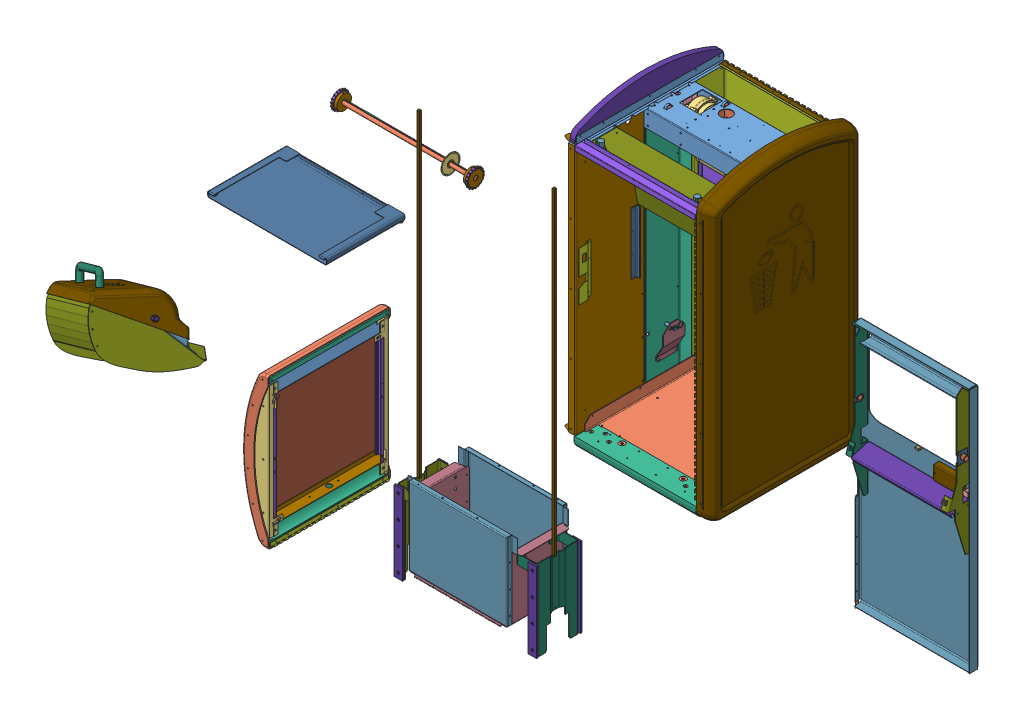
SolidWorks assembly BB3_Assy, configuration Défaut. Lengths in mm.
Overall size (2851.62 1575.75 2038.4).
154 component instances, 91 part files, 0 mates.
Components (placement in the parent):
- BB3_Chassis-1: BB3_Chassis [Défaut] at (-41.1099 482.798 -82.8142) size (675.82 1282.03 663.93)
  - TopCrossmember_Rev2-1: TopCrossmember_Rev2 [Default] at (20.5473 102.5902 0) size (635 86.99 210.82)
  - TopCrossMotorBrkt_Rev3-1: TopCrossMotorBrkt_Rev3 [Défaut] at (-101.9976 61.051 0) size (152.4 200.54 205.51)
  - Moto_Reducteur_011_562_1_216-1: Moto_Reducteur_011_562_1_216 [Default] at (192.9322 74.2423 -36.8146) x (0 -0.000019 -1) z (-1 0 0) size (114.3 226.4 239.81)
  - TopCrossBearingBrkt_Rev1-1: TopCrossBearingBrkt_Rev1 [Défaut] at (-246.0257 61.051 0) size (25.4 73.66 205.51)
  - TopCrossBearingBrkt_Rev1-2: TopCrossBearingBrkt_Rev1 [Défaut] at (287.1203 61.051 0) x (-1 0 0) z (0 0 -1) size (25.4 73.66 205.51)
  - Chassis_Coussinet-1: Chassis_Coussinet [Default] at (-247.5497 60.2788 -36.8146) x (0 -0.995993 0.089436) z (0 0.089436 0.995993) size (28.27 19.05 28.27)
  - Chassis_Coussinet-2: Chassis_Coussinet [Default] at (288.6443 60.2788 -36.8146) x (0 0.997938 0.064185) z (0 -0.064185 0.997938) size (28.27 19.05 28.27)
  - Chassis_Support_Moteur-1: Chassis_Support_Moteur [Défaut] at (-296.9017 100.6288 0.0002) x (0 0 1) z (0 1 0) size (205.51 54 1127)
  - Chassis_Support_Moteur-2: Chassis_Support_Moteur [Défaut] at (337.9963 100.6288 0.0002) x (0 0 -1) z (0 1 0) size (205.51 54 1127)
  - Chassis_Panneau_Arriere-2: Chassis_Panneau_Arriere [Défaut] at (20.5983 -479.4712 -246.619) x (0 0 1) z (0 1 0) size (164.98 667 1155.29)
  - Chassis_Support_Batterie-2: Chassis_Support_Batterie [Défaut] at (20.5983 -270.8192 -242.544) x (0 0 1) z (-1 0 0) size (116.32 446 529)
  - Chassis_Support_Moteur_Devant_Gauche-2: Chassis_Support_Moteur_Devant_Gauche [Défaut] at (-249.8894 -442.8187 130.7585) x (0 0 -1) z (0 1 0) size (329.85 66 1105)
  - Chassis_Positionnement_Emetteur_Recepteur_Gauche-2: Chassis_Positionnement_Emetteur_Recepteur_Gauche [Défaut] at (-222.4622 -381.8185 156.8606) x (1 0 0) z (0 -1 0) size (22.1 48.5 273)
  - Chassis_Support_Moteur_Devant_Droite-1: Chassis_Support_Moteur_Devant_Droite [Défaut] at (290.9839 -442.8187 130.7585) x (0 0 -1) z (0 -1 0) size (329.85 66 1105)
  - Chassis_Positionnement_Emetteur_Recepteur_Droite-1: Chassis_Positionnement_Emetteur_Recepteur_Droite [Défaut] at (263.5568 -381.8185 156.8606) x (-1 0 0) z (0 1 0) size (22.1 48.5 273)
  - Chassis_Support_Pignon_bas-1: Chassis_Support_Pignon_bas [Défaut] at (305.4963 -865.3715 -39.8528) x (-1 0 0) z (0 0 1) size (35.2 151.29 95)
  - Chassis_Axe_Pignon_Bas-1: Chassis_Axe_Pignon_Bas [Défaut] at (340.9963 -816.3715 -39.8528) x (-1 0 0) z (0 -0.052233 -0.998635) size (48.6 15.9 15.9)
  - Chassis_Goupille_Axe_Pignon_bas-1: Chassis_Goupille_Axe_Pignon_bas [Défaut] at (300.5463 -817.6251 -63.8201) x (0 0.052233 0.998635) z (1 0 0) size (60.5 23 3)
  - Chassis_Support_Pignon_bas-2: Chassis_Support_Pignon_bas [Défaut] at (-264.4017 -865.3715 -39.8528) x (1 0 0) z (0 0 -1) size (35.2 151.29 95)
  - Chassis_Axe_Pignon_Bas-2: Chassis_Axe_Pignon_Bas [Défaut] at (-299.9017 -816.3715 -39.8528) x (1 0 0) z (0 0.31653 0.948583) size (48.6 15.9 15.9)
  - Chassis_Goupille_Axe_Pignon_bas-2: Chassis_Goupille_Axe_Pignon_bas [Défaut] at (-259.4517 -808.7748 -17.0869) x (0 -0.31653 -0.948583) z (1 0 0) size (60.5 23 3)
  - Chassis_Plaque_Haute-1: Chassis_Plaque_Haute [Défaut] at (20.4963 92.768 412.6062) x (0 0 -1) z (1 0 0) size (278.51 354.1 562.7)
  - Chassis_Renfort-1: Chassis_Renfort [Défaut] at (20.5463 -1018.8712 0.0002) x (0 0 1) z (-1 0 0) size (199.51 39 641)
  - Chassis_Charniere_Photovoltaique-1: Chassis_Charniere_Photovoltaique [Défaut] at (20.5983 134.4053 -220.1468) x (0 0 -1) z (1 0 0) size (21.77 6 520)
  - Chassis_Equerre_Haute-1: Chassis_Equerre_Haute [Défaut] at (-246.1446 112.2812 81.6782) x (1 0 0.000001) z (-0.000001 0 1) size (44 37.45 648)
  - Chassis_Equerre_Haute-2: Chassis_Equerre_Haute [Défaut] at (287.2893 112.2812 81.6751) x (-1 0 -0.000168) z (0.000168 0 -1) size (44 37.45 648)
  - Chassis_Repose_Bac_Dechets-1: Chassis_Repose_Bac_Dechets [Défaut] at (20.4963 -992.8728 80.2436) x (0 -0.000001 1) z (-1 0 0) size (641.73 77 529)
  - Chassis_Semelle-1: Chassis_Semelle [Défaut] at (20.4963 -1034.3925 80.4561) x (1 0 0) z (0 -0.000001 1) size (404.15 56 558)
  - Chassis_Repose_Pied-1: Chassis_Repose_Pied [Défaut] at (-187.0037 -1049.3185 336.4561) x (1 0 0) z (0 -0.000001 1) size (94 52.5 63.3)
  - Chassis_Repose_Pied-2: Chassis_Repose_Pied [Défaut] at (-187.0037 -1049.3182 -175.5439) x (1 0 0) z (0 -0.000001 1) size (94 52.5 63.3)
  - Chassis_Repose_Pied-3: Chassis_Repose_Pied [Défaut] at (227.9963 -1049.3182 -175.5439) x (1 0 0) z (0 -0.000001 1) size (94 52.5 63.3)
  - Chassis_Repose_Pied-4: Chassis_Repose_Pied [Défaut] at (227.9963 -1049.3185 336.4561) x (1 0 0) z (0 -0.000001 1) size (94 52.5 63.3)
  - Chassis_Repose_Pied_Insert-1: Chassis_Repose_Pied_Insert [Défaut] at (-187.0037 -1050.3185 336.4561) x (0 1 0.000001) z (0.428959 -0.000001 0.903324) size (14.3 17.5 17.5)
  - Chassis_Repose_Pied_Insert-2: Chassis_Repose_Pied_Insert [Défaut] at (227.9963 -1050.3185 336.4561) x (0 1 0.000001) z (0.384049 -0.000001 0.923313) size (14.3 17.5 17.5)
  - Chassis_Repose_Pied_Insert-3: Chassis_Repose_Pied_Insert [Défaut] at (227.9963 -1050.3182 -175.5439) x (0 1 0.000001) z (-0.000001 -0.000001 1) size (14.3 17.5 17.5)
  - Chassis_Repose_Pied_Insert-4: Chassis_Repose_Pied_Insert [Défaut] at (-187.0037 -1050.3182 -175.5439) x (0 1 0.000001) z (-0.000001 -0.000001 1) size (14.3 17.5 17.5)
  - Chassis_Repose_Pied_Insert-5: Chassis_Repose_Pied_Insert [Défaut] at (-114.0037 -995.8185 336.4561) x (0 -1 -0.000001) z (0.798225 0 0.602359) size (14.3 17.5 17.5)
  - Chassis_Repose_Pied_Insert-6: Chassis_Repose_Pied_Insert [Défaut] at (154.9963 -995.8185 336.4561) x (0 -1 -0.000001) z (0.000001 -0.000001 1) size (14.3 17.5 17.5)
  - Chassis_Repose_Pied_Insert-7: Chassis_Repose_Pied_Insert [Défaut] at (-114.0037 -995.8182 -175.5439) x (0 -1 -0.000001) z (0.000001 -0.000001 1) size (14.3 17.5 17.5)
  - Chassis_Repose_Pied_Insert-8: Chassis_Repose_Pied_Insert [Défaut] at (154.9963 -995.8182 -175.5439) x (0 -1 -0.000001) z (0.000001 -0.000001 1) size (14.3 17.5 17.5)
  - Chassis_Dessous_Avant_Porte-1: Chassis_Dessous_Avant_Porte [Défaut] at (20.4963 -992.8728 80.2436) x (0 -0.000001 1) z (-1 0 0) size (98 53.79 536)
  - Chassis_Serrure-1: Chassis_Serrure [Défaut] at (-243.4017 -382.964 366.4072) x (1 0 0) z (0 1 0) size (10.5 63.82 216)
  - Chassis_Equerre_Face-1: Chassis_Equerre_Face [Défaut] at (20.4963 111.0096 411.9878) x (0 0 1) z (-1 0 0) size (32.2 41.42 529)
  - Chassis_Charniere_Support_Moteur_Devant_Droite-1: Chassis_Charniere_Support_Moteur_Devant_Droite [Défaut] at (260.2718 -465.3185 388.412) x (0 0 1) z (0 -1 0) size (21.77 6 1066)
  - Chassis_Serrure_Cle-1: Chassis_Serrure_Cle [Défaut] at (-191.3537 126.1269 363.7894) x (0 1 0) z (-1 0 0) size (41.58 38.56 38.97)
    - Chassis_Serrure_Came-1: Chassis_Serrure_Came [Défaut] at (-18.246 14.5659 16.3878) x (0 -1 0) z (1 0 0) size (12.45 12.01 13.54)
    - Chassis_Serrure_Rondelle_Ecrou-1: Chassis_Serrure_Rondelle_Ecrou [Défaut] at (-31.074 17.7899 -9.8703) x (0 0.096744 0.995309) z (-1 0 0) size (35.31 35.31 0.64)
    - Chassis_Serrure_Ecrou_Hex-1: Chassis_Serrure_Ecrou_Hex [Défaut] at (-26.3115 -31.157 8.2014) x (0 0 1) z (-1 0 0) size (33 28.58 4.76)
    - Chassis_Serrure_Insert_Cle-1: Chassis_Serrure_Insert_Cle [Défaut] at (26.379 -212.8643 14.6) x (-1 0 0) z (0 0 -1) size (23.33 15.95 15.95)
    - Chassis_Serrure_Support-1: Chassis_Serrure_Support [Défaut] at (-26.6815 11.1833 12.473) x (-1 0 0) z (0 -1 0) size (41.46 28.7 28.7)
    - Chassis_Serrure_Ressort-1: Chassis_Serrure_Ressort [Défaut] at (-1.4058 10.243 9.1044) x (0 0 -1) z (1 0 0) size (21.49 4.59 4.57)
    - Chassis_Serrure_Pene-1: Chassis_Serrure_Pene [Défaut] at (1.0072 5.2825 -10.1896) x (0 -0.999973 -0.007317) z (-1 0 0) size (16.91 23.47 9.63)
  - Chassis_Serrure_Cle-2: Chassis_Serrure_Cle [Défaut] at (232.3463 126.1269 341.4229) x (0 1 0) z (1 0 0) size (41.58 38.56 38.97)
    - Chassis_Serrure_Came-1: Chassis_Serrure_Came [Défaut] at (-18.246 14.5659 16.3878) x (0 -1 0) z (1 0 0) size (12.45 12.01 13.54)
    - Chassis_Serrure_Rondelle_Ecrou-1: Chassis_Serrure_Rondelle_Ecrou [Défaut] at (-31.074 17.7899 -9.8703) x (0 0.096744 0.995309) z (-1 0 0) size (35.31 35.31 0.64)
    - Chassis_Serrure_Ecrou_Hex-1: Chassis_Serrure_Ecrou_Hex [Défaut] at (-26.3115 -31.157 8.2014) x (0 0 1) z (-1 0 0) size (33 28.58 4.76)
    - Chassis_Serrure_Insert_Cle-1: Chassis_Serrure_Insert_Cle [Défaut] at (26.379 -212.8643 14.6) x (-1 0 0) z (0 0 -1) size (23.33 15.95 15.95)
    - Chassis_Serrure_Support-1: Chassis_Serrure_Support [Défaut] at (-26.6815 11.1833 12.473) x (-1 0 0) z (0 -1 0) size (41.46 28.7 28.7)
    - Chassis_Serrure_Ressort-1: Chassis_Serrure_Ressort [Défaut] at (-1.4058 10.243 9.1044) x (0 0 -1) z (1 0 0) size (21.49 4.59 4.57)
    - Chassis_Serrure_Pene-1: Chassis_Serrure_Pene [Défaut] at (1.0072 5.2825 -10.1896) x (0 -0.999973 -0.007317) z (-1 0 0) size (16.91 23.47 9.63)
  - Tombstone_Rev1-1: Tombstone_Rev1 [Default] at (288.5894 129.5652 81.0473) x (1 0 0.000168) z (-0.000168 0 1) size (22.23 105.62 654.05)
  - Tombstone_Rev1-2: Tombstone_Rev1 [Default] at (-247.4446 129.5652 82.3062) x (-1 0 -0.000001) z (0.000001 0 -1) size (22.23 105.62 654.05)
  - SideSkin_Rev1-1: SideSkin_Rev1 [Default] at (-317.3073 -1045.6118 82.3061) x (-1 0 -0.000001) z (0.000001 0 -1) size (69.87 1274.83 660.4) (hidden)
  - SideSkin_Rev1-2: SideSkin_Rev1 [Default] at (358.4521 -1045.6118 81.059) x (1 0 0.000168) z (-0.000168 0 1) size (69.87 1274.83 660.4)
  - Chassis_Interieur_Cache_Chaine-1: Chassis_Interieur_Cache_Chaine [Défaut] at (-242.9017 -763.8184 0) x (0 -0.000001 1) z (-1 0 0) size (249 989 21) (hidden)
  - Chassis_Interieur_Cache_Chaine-2: Chassis_Interieur_Cache_Chaine [Défaut] at (283.9963 -763.8185 0.0002) x (0 0 -1) z (1 0 0) size (249 989 21)
  - Chassis_Bac_Dechets-1: Chassis_Bac_Dechets [Défaut] at (19.5983 -711.9931 65.1059) x (-1 0 0) z (0 0.000001 -1) size (517 387.96 620.45) (hidden)
- BB3_Axe_Moteur-1: BB3_Axe_Moteur [Défaut] at (-1009.5034 267.4996 345.1119) size (601.11 82.55 82.55)
  - TransmissionShaft_Rev1-1: TransmissionShaft_Rev1 [Défaut] at (-0.7672 -0.3857 -1.9336) size (596.9 18.75 19.05)
  - CounterDisc_Rev1-1: CounterDisc_Rev1 [Défaut] at (188.8209 -0.3857 -1.9336) size (0.91 82.55 82.55)
  - Pignon_Haut-1: Pignon_Haut [Défaut] at (-297.0312 -0.3857 -1.9336) x (0 0 1) z (-1 0 0) (suppressed, hidden)
  - Pignon_Haut-2: Pignon_Haut [Défaut] at (294.0828 -0.3857 -1.9336) x (0 0 -1) z (1 0 0) (suppressed, hidden)
  - SHAFT_COLLAR_MCMASTER_6166K28-1: SHAFT_COLLAR_MCMASTER_6166K28 [Défaut] at (181.6772 -0.3857 -1.9336) size (14.29 38.1 38.1)
  - TRANSMISSION_KEY_MC_98870A140-1: TRANSMISSION_KEY_MC_98870A140 [Défaut] at (-285.8172 18.6654 -1.9336) x (-1 0 0) z (0 0 1) size (25.4 4.76 4.76)
  - TRANSMISSION_KEY_MC_98870A140-2: TRANSMISSION_KEY_MC_98870A140 [Défaut] at (284.2828 18.6654 -1.9336) x (-1 0 0) z (0 0 1) size (25.4 4.76 4.76)
  - TRANSMISSION_KEY_MC_98870A190-1: TRANSMISSION_KEY_MC_98870A190 [Défaut] at (-155.0672 18.6654 -1.9336) x (-1 0 0) z (0 0 1) size (63.5 4.76 4.76)
  - PURPLE_IGUS-1: PURPLE_IGUS [Défaut] at (191.2568 -0.3857 -1.9336) x (0 0.381849 -0.924225) z (0 0.924225 0.381849) size (28.27 19.05 28.27)
  - BB3_Pignon_Cylindre_Primitif-1: BB3_Pignon_Cylindre_Primitif [Défaut] at (-295.6312 -0.3857 -1.9336) x (0 0 -1) z (1 0 0) size (73.14 73.14 10)
  - BB3_Pignon_Cylindre_Primitif-2: BB3_Pignon_Cylindre_Primitif [Défaut] at (295.4828 -0.3857 -1.9336) x (0 0 -1) z (1 0 0) size (73.14 73.14 10)
  - Pignon_Haut-3: Pignon_Haut [Défaut] at (-297.0312 -0.3857 -1.9336) x (0 0 1) z (-1 0 0)
  - Pignon_Haut-4: Pignon_Haut [Défaut] at (296.8828 -0.3857 -1.9336) x (0 0 -1) z (1 0 0)
- BB3_Coulissant_Vertical-1: BB3_Coulissant_Vertical [Défaut] at (-1026.0534 143.9476 740.0072) size (524 38.71 350.2)
  - Plaque_Coulissante-1: Plaque_Coulissante [Défaut] at (-32.873 42.5619 -174.4999) size (524 25.8 349)
  - Butoir_Haut-1: Butoir_Haut [Défaut] at (-32.873 49.4619 -175.6999) x (0 -1 0) z (1 0 0) size (32.71 10.73 508)
- BB3_Dévidoir-1: BB3_Dévidoir [Défaut] at (-1393.6514 -79.7778 1289.016) size (642 556.94 573.94)
  - HopperRollRod_Rev3-1: HopperRollRod_Rev3 [Default] at (155.8236 65.6237 286.0909) x (0.795138 0.485459 0.363434) z (-0.19783 0.774165 -0.601275) size (428.62 9.53 9.53)
  - PEM-FH-0420-20-1: PEM-FH-0420-20 [Default] at (393.3249 56.2024 61.1725) x (0.795138 0.485459 0.363434) z (-0.606428 0.636526 0.476529) size (8.56 31.75 8.56)
  - PEM-FH-0420-20-2: PEM-FH-0420-20 [Default] at (231.7529 -42.443 -12.6774) x (0.795138 0.485459 0.363434) z (-0.606428 0.636526 0.476529) size (8.56 31.75 8.56)
  - DoorShield_Rev2-2: DoorShield_Rev2 [Default] at (302.6515 19.535 28.9751) x (-0.795138 -0.485459 -0.363434) z (0.606428 -0.636526 -0.476529) size (434.07 74.67 214.39)
  - HANDLE_MC_1435A43-1: HANDLE_MC_1435A43 [Default] at (121.4778 196.7862 188.5909) x (-0.795138 -0.485459 -0.363434) z (-0.363434 0.861227 -0.355251) size (228.6 25.4 88.9)
  - HopperBase_Rev1-2: HopperBase_Rev1 [Default] at (116.9003 195.0314 200.9498) x (-0.795138 -0.485459 -0.363434) z (-0.363434 0.861227 -0.355251) size (431.8 386.04 237.96)
  - HopperRod_Rev3-3: HopperRod_Rev3 [Default] at (213.8333 117.6327 92.2617) x (0.795138 0.485459 0.363434) z (-0.363434 -0.098284 0.926421) size (482.6 19.05 19.05)
  - HopperSkin_Rev1-2: HopperSkin_Rev1 [Default] at (213.8331 117.6327 92.2616) x (-0.795138 -0.485459 -0.363434) z (-0.172906 0.755914 -0.631424) size (450.64 354.33 119.73)
  - HopperCounterweight_Rev3-1: HopperCounterweight_Rev3 [Default] at (312.5389 13.9139 14.8515) x (0.795138 0.485459 0.363434) z (0.606428 -0.636526 -0.476529) size (251.46 15.88 25.4)
- BB3_Panneau_Solaire-1: BB3_Panneau_Solaire [Défaut] at (-458.5936 -250.3477 1146.6516) size (123.03 660.4 537.47)
  - Panneau_Polycarbonate-1: Panneau_Polycarbonate [Défaut] at (-125.4878 -275.8438 -268.7327) size (113.53 660.4 537.47)
  - Panneau_Support_Latéral-1: Panneau_Support_Latéral [Défaut] at (-148.4298 46.843 -263.9327) size (113.03 640.4 62.5)
  - Panneau_Support_Latéral-2: Panneau_Support_Latéral [Défaut] at (-148.4298 46.843 263.9327) x (1 0 0) z (0 0 -1) size (113.03 640.4 62.5)
  - Panneau_Support_Insert-1: Panneau_Support_Insert [Défaut] at (-150.3855 -359.157 263.9327) x (-1 0 0) z (0 0 1) size (6 6.93 1.6)
  - Panneau_Support_Insert-2: Panneau_Support_Insert [Défaut] at (-85.828 452.843 263.9327) size (6 6.93 1.6)
  - Panneau_Support_Insert-3: Panneau_Support_Insert [Défaut] at (41.5571 -82.6112 263.9327) x (-0.5 -0.866025 0) z (0 0 1) size (6 6.93 1.6)
  - Panneau_Support_Insert-4: Panneau_Support_Insert [Défaut] at (-277.7705 -82.6112 -263.9327) x (0.5 -0.866025 0) z (0 0 -1) size (6 6.93 1.6)
  - Panneau_Support_Insert-5: Panneau_Support_Insert [Défaut] at (73.8358 -229.7028 -263.9327) x (0.5 0.866025 0) z (0 0 -1) size (6 6.93 1.6)
  - Panneau_Support_Insert-6: Panneau_Support_Insert [Défaut] at (-85.828 46.843 -263.9327) x (1 0 0) z (0 0 -1) size (6 6.93 1.6)
  - Panneau_Support_Insert_Axe-1: Panneau_Support_Insert_Axe [Défaut] at (-134.2461 221.8888 -263.5327) x (0.5 0.866025 0) z (0 0 1) size (5 5 6)
  - Panneau_Support_Insert_Axe-2: Panneau_Support_Insert_Axe [Défaut] at (-85.8495 -154.978 -263.5327) x (-0.999333 -0.036528 0) z (0 0 1) size (5 5 6)
  - Panneau_Support_Insert_Axe-3: Panneau_Support_Insert_Axe [Défaut] at (-147.9235 34.4786 263.5327) x (0.923728 0.383049 0) z (0 0 -1) size (5 5 6)
  - Panneau_Support_Insert_Axe-4: Panneau_Support_Insert_Axe [Défaut] at (-88.29 262.2073 263.5327) x (-0.923728 -0.383049 0) z (0 0 -1) size (5 5 6)
  - Panneau_Support_Insert_Axe-5: Panneau_Support_Insert_Axe [Défaut] at (-88.29 -143.7927 263.5327) x (-0.923728 -0.383049 0) z (0 0 -1) size (5 5 6)
  - Panneau_Support_Insert_Axe-6: Panneau_Support_Insert_Axe [Défaut] at (-114.6975 14.7448 -263.5327) x (-0.105618 0.994407 0) z (0 0 1) size (5 5 6)
  - Panneau_Support_Photovoltaique-1: Panneau_Support_Photovoltaique [Défaut] at (-129.7625 46.843 -262.4327) size (63.24 656.65 524.87)
  - Panneau_Charnière-1: Panneau_Charnière [Défaut] at (-66.9385 -256.8848 -0.0002) x (0 -1 0) z (0 0 1) size (21.77 6 520)
  - Panneau_Profilé_Photovoltaique-1: Panneau_Profilé_Photovoltaique [Défaut] at (-116.513 46.843 -244.0327) x (0 0 1) z (0 -1 0) size (27 50 494)
  - Panneau_Profilé_Photovoltaique-2: Panneau_Profilé_Photovoltaique [Défaut] at (-116.513 46.843 244.0327) x (0 0 -1) z (0 1 0) size (27 50 494)
  - Panneau_Profilé2_Photovoltaique-1: Panneau_Profilé2_Photovoltaique [Défaut] at (-159.6417 81.843 0) x (-1 0 0) z (0 0 1) size (50 18.97 515.06)
  - Panneau_Profilé3_Photovoltaique-1: Panneau_Profilé3_Photovoltaique [Défaut] at (-159.6417 11.843 0) x (-1 0 0) z (0 0 -1) size (50 18.97 515.06)
  - Panneau_Photovoltaique-1: Panneau_Photovoltaique [Défaut] at (-140.313 46.843 -0.0002) x (0 0 -1) z (1 0 0) size (512.06 494 5.7)
  - Panneau_Digital-1: Panneau_Digital [Défaut] at (-122.5314 44.8723 0.0023) x (0.063139 -0.998005 0) z (0 0 -1) size (25.38 29.97 80)
  - Panneau_Jambe-1: Panneau_Jambe [Défaut] at (-87.1789 273.5009 248.1827) x (0.999999 -0.001582 0) z (-0.001582 -0.999999 0) size (22.02 30.02 480.49)
- BB3_Porte-1: BB3_Porte [Défaut] at (895.8135 -255.8374 27.3656) size (899.17 1120.24 468.39)
  - Porte_Devant-1: Porte_Devant [Défaut] at (265.4153 -39.6917 -280.2063) size (521.6 1080.12 53)
  - Porte_Plaque_Support_Devidoir_Droite-1: Porte_Plaque_Support_Devidoir_Droite [Défaut] at (-239.7055 206.7117 47.939) x (0.939693 -0.321394 0.116978) z (0.34202 0.883022 -0.321394) size (245.58 270.63 576.7)
  - Porte_Plaque_Support_Devidoir_Gauche-1: Porte_Plaque_Support_Devidoir_Gauche [Défaut] at (253.7381 206.7117 47.939) x (-0.939693 -0.321394 0.116978) z (0.34202 -0.883022 0.321394) size (235.72 270.63 576.7)
  - Porte_Plaque_Support_Devidoir_Centre-1: Porte_Plaque_Support_Devidoir_Centre [Défaut] at (7.0162 30.6943 16.6558) x (0 -0.258819 0.965926) z (-1 0 0) size (85.71 18.5 445.2)
  - Porte_Poignee_Arriere-1: Porte_Poignee_Arriere [Défaut] at (150.1174 92.5415 -24.8999) x (1 0 0) z (0 1 0) size (121.4 25.4 64.3)
  - Porte_Poignee_Devant-1: Porte_Poignee_Devant [Défaut] at (150.1174 85.2415 -2.5999) x (1 0 0) z (0 1 0) size (122.99 27.13 46.9)
  - Porte_Charniere-1: Porte_Charniere [Défaut] at (-277.2955 -54.1847 3.3348) x (-0.173648 0 -0.984808) z (0 1 0) size (21.77 6 1092)
  - Porte_Serrure_Cle-1: Porte_Serrure_Cle [Défaut] at (242.4153 102.2755 6.859) x (0 0 1) z (1 0 0) size (41.58 38.56 38.97)
    - Porte_Serrure_Ressort-1: Porte_Serrure_Ressort [Défaut] at (-1.4058 10.243 9.1044) x (0 0 -1) z (1 0 0) size (21.49 4.59 4.57)
    - Porte_Serrure_Support-1: Porte_Serrure_Support [Défaut] at (-26.6815 11.1833 12.473) x (-1 0 0) z (0 -1 0) size (41.46 28.7 28.7)
    - Porte_Serrure_Insert_Cle-1: Porte_Serrure_Insert_Cle [Défaut] at (26.379 -212.8643 14.6) x (-1 0 0) z (0 0 -1) size (23.33 15.95 15.95)
    - Porte_Serrure_Ecrou_Hex-1: Porte_Serrure_Ecrou_Hex [Défaut] at (-26.3115 -31.157 8.2014) x (0 0 1) z (-1 0 0) size (33 28.58 4.76)
    - Porte_Serrure_Rondelle_Ecrou-1: Porte_Serrure_Rondelle_Ecrou [Défaut] at (-31.074 17.7899 -9.8703) x (0 0.096744 0.995309) z (-1 0 0) size (35.31 35.31 0.64)
    - Porte_Serrure_Came-1: Porte_Serrure_Came [Défaut] at (-18.246 14.5659 16.3878) x (0 -1 0) z (1 0 0) size (12.45 12.01 13.54)
    - Porte_Serrure_Pene-1: Porte_Serrure_Pene [Défaut] at (1.0072 5.2825 -10.1896) x (0 -0.999973 -0.007317) z (-1 0 0) size (16.91 23.47 9.63)
  - Porte_Support_Devidoir-1: Porte_Support_Devidoir [Défaut] at (-219.5828 230.7583 15.6101) x (0 0 1) z (1 0 0) size (44 50 2)
  - Porte_Support_Devidoir-2: Porte_Support_Devidoir [Défaut] at (233.6153 230.7583 15.6101) x (0 0 1) z (-1 0 0) size (44 50 2)
  - Porte_Coussinet-1: Porte_Coussinet [Défaut] at (-217.0588 230.7583 12.6101) x (0 0.383049 -0.923728) z (0 0.923728 0.383049) size (28.27 19.05 28.27)
  - Porte_Coussinet-2: Porte_Coussinet [Défaut] at (231.0913 230.7583 12.6101) x (0 0.383049 0.923728) z (0 0.923728 -0.383049) size (28.27 19.05 28.27)
  - Porte_Plaque_Support_Devidoir_Gauche_simulation-1: Porte_Plaque_Support_Devidoir_Gauche_simulation [Défaut] at (214.5427 74.8366 69.753) x (-1 0 0) z (0 0.34202 0.939693) size (15.52 15.52 7.76)
  - Porte_Plaque_Support_Devidoir_Gauche_simulation-2: Porte_Plaque_Support_Devidoir_Gauche_simulation [Défaut] at (7.0173 130.9233 -18.7399) x (1 0 0) z (0 1 0) size (15.52 15.52 7.76)
- BB3_Rame_Compacteur-1: BB3_Rame_Compacteur [Défaut] at (-210.6832 -662.3995 814.6271) size (627.3 1739.7 268.31)
  - Compacteur_Rame-1: Compacteur_Rame [Défaut] at (24.383 25.4321 -2.9042) size (505.8 287.44 265.81)
  - Compacteur_Flasque-1: Compacteur_Flasque [Défaut] at (23.883 58.9321 129.5958) x (-1 0 0) z (0 0 -1) size (481.4 343 21.8)
  - Compacteur_Flasque-2: Compacteur_Flasque [Défaut] at (24.883 58.9321 -135.4042) size (481.4 343 21.8)
  - Compacteur_Guide_Droit-1: Compacteur_Guide_Droit [Défaut] at (297.583 154.6611 -2.9042) x (0 0 1) z (0 -1 0) size (185.61 92.3 356)
  - Compacteur_Guide_Gauche-1: Compacteur_Guide_Gauche [Défaut] at (-250.117 154.6611 -2.9042) x (0 0 -1) z (0 -1 0) size (185.61 93.6 356)
  - Compacteur_Guide_Patin-1: Compacteur_Guide_Patin [Défaut] at (-270.917 -23.3389 -95.7102) x (-1 0 0) z (0 0 -1) size (38 350 6.7)
  - Compacteur_Guide_Patin-2: Compacteur_Guide_Patin [Défaut] at (-270.917 -23.3389 89.9018) size (38 350 6.7)
  - Compacteur_Guide_Patin-3: Compacteur_Guide_Patin [Défaut] at (318.383 -23.3389 89.9018) size (38 350 6.7)
  - Compacteur_Guide_Patin-4: Compacteur_Guide_Patin [Défaut] at (318.383 -23.3389 -95.7102) x (-1 0 0) z (0 0 -1) size (38 350 6.7)
  - BB3_Coulissant_Vertical_Cremaillere-1: BB3_Coulissant_Vertical_Cremaillere [Défaut] at (-273.2835 838.3611 2.0958) x (-1 0 0) z (0 -1 0) size (10 10 1400)
  - BB3_Coulissant_Vertical_Cremaillere-2: BB3_Coulissant_Vertical_Cremaillere [Défaut] at (320.7496 838.3611 2.0958) x (1 0 0) z (0 1 0) size (10 10 1400)
